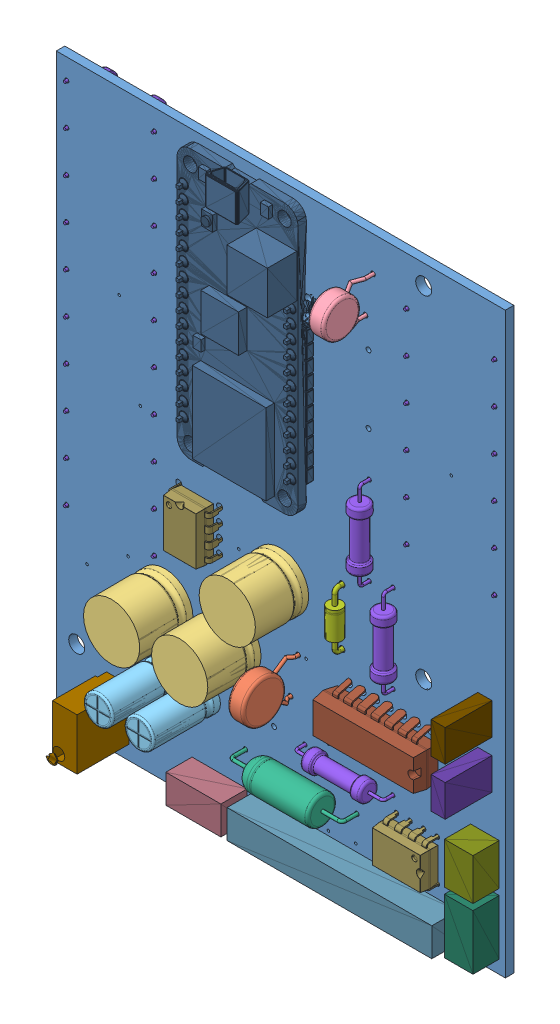
SolidWorks assembly SHEIKAHSLATE, configuration Default. Lengths in mm.
Overall size (83.82 111.16 36.76).
44 component instances, 18 part files, 0 mates.
Components (placement in the parent):
- Board_SHEIKAHSLATE-1: Board_SHEIKAHSLATE [Default] at origin size (83.82 107.95 1.59)
- HAU470KBAUARKR-1: HAU470KBAUARKR [Default] at (53.34 12.7 0.05) x (0 1 0) z (0 0 1) size (8 3 13.01)
- MALREKA00DE433BG0K-1: MALREKA00DE433BG0K [Default] at (50.8 26.83 0.05) x (0 1 0) z (0 0 1) size (10.51 10.5 11.95)
- MALREKA00DE433BG0K-2: MALREKA00DE433BG0K [Default] at (29.21 12.7 0.05) size (10.51 10.5 11.95)
- MALREKA00DE433BG0K-3: MALREKA00DE433BG0K [Default] at (41.91 12.7 0.05) size (10.51 10.5 11.95)
- A102J15C0GF5UAAP-1: A102J15C0GF5UAAP [Default] at (67.31 81.28 0.05) x (0 -1 0) z (0 0 1) size (7.99 3 12.01)
- Noname_1-1: Noname_1 [Default] at (36.83 1.27 0.05) size (5.5 5.5 14.5)
- Noname_1-2: Noname_1 [Default] at (29.21 1.27 0.05) size (5.5 5.5 14.5)
- TVA1161-1: TVA1161 [Default] at (54.61 -3.81 0.05) size (21.4 5.51 7.51)
- 1N5819G-1: 1N5819G [Default] at (62.23 26.67 0) x (0 -1 0) z (0 0 1) size (11.27 2.71 4.71)
- Noname_2-1: Noname_2 [Default] at (67.31 43.18 0) x (0 -1 0) z (0 0 1) size (16.91 3.6 5.6)
- Noname_2-2: Noname_2 [Default] at (46.99 58.42 -1.5896) x (0 1 0) z (0 0 -1) size (16.91 3.6 5.6)
- Noname_2-3: Noname_2 [Default] at (19.05 87.63 -1.5896) x (-1 0 0) z (0 0 -1) size (16.91 3.6 5.6)
- Noname_2-4: Noname_2 [Default] at (19.05 80.01 -1.5896) x (-1 0 0) z (0 0 -1) size (16.91 3.6 5.6)
- Noname_2-5: Noname_2 [Default] at (19.05 72.39 -1.5896) x (-1 0 0) z (0 0 -1) size (16.91 3.6 5.6)
- Noname_2-6: Noname_2 [Default] at (19.05 64.77 -1.5896) x (-1 0 0) z (0 0 -1) size (16.91 3.6 5.6)
- Noname_2-7: Noname_2 [Default] at (19.05 57.15 -1.5896) x (-1 0 0) z (0 0 -1) size (16.91 3.6 5.6)
- Noname_2-8: Noname_2 [Default] at (19.05 49.53 -1.5896) x (-1 0 0) z (0 0 -1) size (16.91 3.6 5.6)
- Noname_2-9: Noname_2 [Default] at (19.05 41.91 -1.5896) x (-1 0 0) z (0 0 -1) size (16.91 3.6 5.6)
- Noname_2-10: Noname_2 [Default] at (19.05 34.29 -1.5896) x (-1 0 0) z (0 0 -1) size (16.91 3.6 5.6)
- Noname_2-11: Noname_2 [Default] at (19.05 26.67 -1.5896) x (-1 0 0) z (0 0 -1) size (16.91 3.6 5.6)
- Noname_2-12: Noname_2 [Default] at (19.05 19.05 -1.5896) x (-1 0 0) z (0 0 -1) size (16.91 3.6 5.6)
- Noname_2-13: Noname_2 [Default] at (82.55 44.45 -1.5896) x (1 0 0) z (0 0 -1) size (16.91 3.6 5.6)
- Noname_2-14: Noname_2 [Default] at (82.55 52.07 -1.5896) x (1 0 0) z (0 0 -1) size (16.91 3.6 5.6)
- Noname_2-15: Noname_2 [Default] at (82.55 59.69 -1.5896) x (1 0 0) z (0 0 -1) size (16.91 3.6 5.6)
- Noname_2-16: Noname_2 [Default] at (82.55 67.31 -1.5896) x (1 0 0) z (0 0 -1) size (16.91 3.6 5.6)
- Noname_2-17: Noname_2 [Default] at (82.55 74.93 -1.5896) x (1 0 0) z (0 0 -1) size (16.91 3.6 5.6)
- Noname_2-18: Noname_2 [Default] at (82.55 82.55 -1.5896) x (1 0 0) z (0 0 -1) size (16.91 3.6 5.6)
- Noname_2-19: Noname_2 [Default] at (48.26 78.74 -1.5896) x (0 -1 0) z (0 0 -1) size (16.91 3.6 5.6)
- Noname_2-20: Noname_2 [Default] at (39.37 78.74 -1.5896) x (0 1 0) z (0 0 -1) size (16.91 3.6 5.6)
- Noname_2-21: Noname_2 [Default] at (71.755 27.94 0) x (0 1 0) z (0 0 1) size (16.91 3.6 5.6)
- Noname_2-22: Noname_2 [Default] at (39.37 58.42 -1.5896) x (0 1 0) z (0 0 -1) size (16.91 3.6 5.6)
- Noname_2-23: Noname_2 [Default] at (63.5 2.54 0) size (16.91 3.6 5.6)
- T93YA-1: T93YA [Default] at (20.32 -13.69 5) size (12.52 14.14 22.04)
- Adafruit_Feather_M0_Adalogger-1: Adafruit_Feather_M0_Adalogger [Default] at (45.72 66.04 3) x (0 -1 0) z (0 0 1) size (54.99 41.16 36.76)
- SN74HC125N-1: SN74HC125N [Default] at (71.24 12.69 0) x (-1 0 0) z (0 1 0) size (19.31 8.27 10.93)
- DIP8-1: DIP8 [Default] at (76.2 -3.81 0) size (15.36 12.48 12.48)
- DIP8-2: DIP8 [Default] at (35.77 29 0) x (0 1 0) z (0 0 1) size (15.36 12.48 12.48)
- 640453-4-1: 640453-4 [Default] at (39.1318 -16.4465 0) size (10.3 5.34 4.91)
- 1-640453-5-1: 1-640453-5 [Default] at (64.53 -16.4465 0) size (38.24 5.34 4.91)
- 640453-4-0-1: 640453-4-0 [Default] at (92.6465 -9.1282 0) x (0 1 0) z (0 0 1) size (10.3 5.34 4.91)
- 640453-3-1: 640453-3 [Default] at (92.6465 1.0303 0) x (-0.000018 1 0) z (0 0 1) size (7.76 5.34 4.91)
- PPTC021LFBN-RC-1: PPTC021LFBN-RC [Default] at (88.689 15.24 0) x (0 1 0) z (0 0 1) size (5.94 2.66 8.76)
- PPTC021LFBN-RC-1-1: PPTC021LFBN-RC-1 [Default] at (88.689 24.13 0) x (-0.000018 1 0) z (0 0 1) size (5.94 2.66 8.76)
